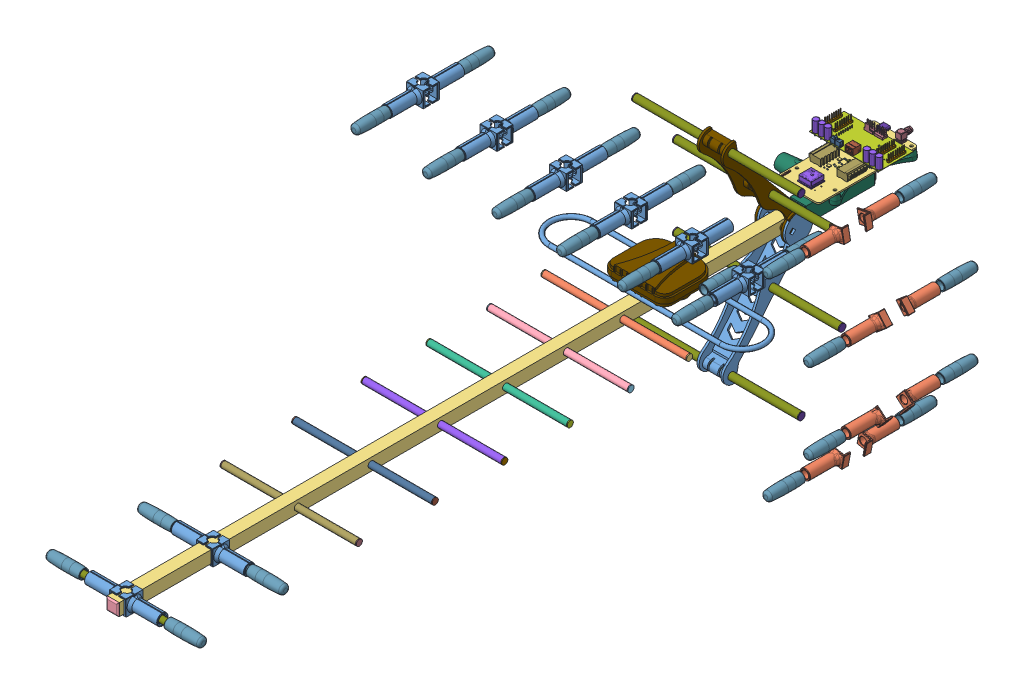
SolidWorks assembly 1. 868MHz Yagi Assembly, configuration Default. Lengths in mm. (continued)
Mates (geometry in assembly coordinates): (continued)
- Concentric20: concentric aligned: cylinder of naked_antenna_v1.step-1/2nd element.step-1/extrusion (2).step-1 through (440.0614 466.1407 645.9384) axis (0 0 1) radius 3.5; cylinder of antenna sheath-20 through (440.0614 466.1407 603.9384) axis (0 0 1) radius 4
- Concentric21: concentric aligned: cylinder of naked_antenna_v1.step-1/3rd element.step-1/extrusion (3).step-1 through (370.0614 466.1407 645.9384) axis (0 0 1) radius 3.5; cylinder of antenna sheath-21 through (370.0614 466.1407 603.9384) axis (0 0 1) radius 4
- Concentric22: concentric aligned: cylinder of naked_antenna_v1.step-1/3rd element.step-1/extrusion (3).step-1 through (370.0614 466.1407 645.9384) axis (0 0 1) radius 3.5; cylinder of antenna sheath-22 through (370.0614 466.1407 603.9384) axis (0 0 1) radius 4
- Concentric23: concentric aligned: cylinder of naked_antenna_v1.step-1/4th element.step-1/extrusion (4).step-1 through (295.0614 466.1407 645.9384) axis (0 0 1) radius 3.5; cylinder of antenna sheath-23 through (295.0614 466.1407 603.9384) axis (0 0 1) radius 4
- Concentric24: concentric aligned: cylinder of naked_antenna_v1.step-1/4th element.step-1/extrusion (4).step-1 through (295.0614 466.1407 645.9384) axis (0 0 1) radius 3.5; cylinder of antenna sheath-24 through (295.0614 466.1407 603.9384) axis (0 0 1) radius 4
- Concentric25: concentric aligned: cylinder of naked_antenna_v1.step-1/5th element.step-1/extrusion (5).step-1 through (215.0614 466.1407 645.9384) axis (0 0 1) radius 3.5; cylinder of antenna sheath-25 through (215.0614 466.1407 603.9384) axis (0 0 1) radius 4
- Concentric26: concentric aligned: cylinder of naked_antenna_v1.step-1/5th element.step-1/extrusion (5).step-1 through (215.0614 466.1407 645.9384) axis (0 0 1) radius 3.5; cylinder of antenna sheath-26 through (215.0614 466.1407 603.9384) axis (0 0 1) radius 4
- Concentric27: concentric aligned: cylinder of naked_antenna_v1.step-1/6th element.step-1/extrusion (6).step-1 through (130.0614 466.1407 645.9384) axis (0 0 1) radius 3.5; cylinder of antenna sheath-27 through (130.0614 466.1407 603.9384) axis (0 0 1) radius 4
- Concentric28: concentric aligned: cylinder of naked_antenna_v1.step-1/6th element.step-1/extrusion (6).step-1 through (130.0614 466.1407 645.9384) axis (0 0 1) radius 3.5; cylinder of antenna sheath-28 through (130.0614 466.1407 603.9384) axis (0 0 1) radius 4
- Concentric29: concentric aligned: cylinder of naked_antenna_v1.step-1/7th element.step-1/extrusion (7).step-1 through (40.0614 466.1407 645.9384) axis (0 0 1) radius 3.5; cylinder of antenna sheath-29 through (-42 0 757.5) axis (1 0 0) radius 4
- Concentric30: concentric aligned: cylinder of naked_antenna_v1.step-1/7th element.step-1/extrusion (7).step-1 through (40.0614 466.1407 645.9384) axis (0 0 1) radius 3.5; cylinder of antenna sheath-30 through (-42 0 757.5) axis (1 0 0) radius 4
- Concentric31: concentric aligned: cylinder of naked_antenna_v1.step-1/8th element.step-1/extrusion (8).step-1 through (-59.9386 466.1407 645.9384) axis (0 0 1) radius 3.5; cylinder of antenna sheath-31 through (-42 0 857.5) axis (1 0 0) radius 4
- Concentric32: concentric aligned: cylinder of naked_antenna_v1.step-1/8th element.step-1/extrusion (8).step-1 through (-59.9386 466.1407 645.9384) axis (0 0 1) radius 3.5; cylinder of antenna sheath-32 through (-42 0 857.5) axis (1 0 0) radius 4
- Coincident9: coincident anti-aligned: plane of naked_antenna_v1.step-1/Extrusion.step-1 through (754.5614 473.1407 652.9384) normal (0 0 1); plane of antenna sheath-3 through (440.0614 466.1407 652.9384) normal (0 0 -1)
- Coincident10: coincident anti-aligned: plane of naked_antenna_v1.step-1/Extrusion.step-1 through (754.5614 473.1407 652.9384) normal (0 0 1); plane of antenna sheath-4 through (440.0614 466.1407 652.9384) normal (0 0 -1)
- Coincident11: coincident anti-aligned: plane of naked_antenna_v1.step-1/Extrusion.step-1 through (754.5614 473.1407 652.9384) normal (0 0 1); plane of antenna sheath-5 through (370.0614 466.1407 652.9384) normal (0 0 -1)
- Coincident12: coincident anti-aligned: plane of naked_antenna_v1.step-1/Extrusion.step-1 through (754.5614 473.1407 652.9384) normal (0 0 1); plane of antenna sheath-6 through (370.0614 466.1407 652.9384) normal (0 0 -1)
- Coincident13: coincident anti-aligned: plane of naked_antenna_v1.step-1/Extrusion.step-1 through (754.5614 473.1407 652.9384) normal (0 0 1); plane of antenna sheath-7 through (295.0614 466.1407 652.9384) normal (0 0 -1)
- Coincident14: coincident anti-aligned: plane of naked_antenna_v1.step-1/Extrusion.step-1 through (754.5614 473.1407 652.9384) normal (0 0 1); plane of antenna sheath-8 through (295.0614 466.1407 652.9384) normal (0 0 -1)
- Coincident15: coincident anti-aligned: plane of naked_antenna_v1.step-1/Extrusion.step-1 through (754.5614 473.1407 652.9384) normal (0 0 1); plane of antenna sheath-9 through (215.0614 466.1407 652.9384) normal (0 0 -1)
- Coincident16: coincident anti-aligned: plane of naked_antenna_v1.step-1/Extrusion.step-1 through (754.5614 473.1407 652.9384) normal (0 0 1); plane of antenna sheath-10 through (215.0614 466.1407 652.9384) normal (0 0 -1)
- Coincident17: coincident anti-aligned: plane of naked_antenna_v1.step-1/Extrusion.step-1 through (754.5614 473.1407 652.9384) normal (0 0 1); plane of antenna sheath-11 through (130.0614 466.1407 652.9384) normal (0 0 -1)
- Coincident18: coincident anti-aligned: plane of naked_antenna_v1.step-1/Extrusion.step-1 through (754.5614 473.1407 652.9384) normal (0 0 1); plane of antenna sheath-12 through (130.0614 466.1407 652.9384) normal (0 0 -1)
- Coincident19: coincident anti-aligned: plane of naked_antenna_v1.step-1/Extrusion.step-1 through (754.5614 473.1407 652.9384) normal (0 0 1); plane of antenna sheath-13 through (40.0614 466.1407 652.9384) normal (0 0 -1)
- Coincident20: coincident anti-aligned: plane of naked_antenna_v1.step-1/Extrusion.step-1 through (754.5614 473.1407 652.9384) normal (0 0 1); plane of antenna sheath-14 through (40.0614 466.1407 652.9384) normal (0 0 -1)
- Coincident21: coincident anti-aligned: plane of naked_antenna_v1.step-1/Extrusion.step-1 through (754.5614 473.1407 652.9384) normal (0 0 1); plane of antenna sheath-15 through (-59.9386 466.1407 652.9384) normal (0 0 -1)
- Coincident22: coincident anti-aligned: plane of naked_antenna_v1.step-1/Extrusion.step-1 through (754.5614 473.1407 652.9384) normal (0 0 1); plane of antenna sheath-16 through (-59.9386 466.1407 652.9384) normal (0 0 -1)
- Coincident23: coincident anti-aligned: plane of naked_antenna_v1.step-1/Extrusion.step-1 through (754.5614 459.1407 638.9384) normal (0 0 -1); plane of antenna sheath-32 through (-59.9386 466.1407 638.9384) normal (0 0 1)
- Coincident24: coincident anti-aligned: plane of naked_antenna_v1.step-1/Extrusion.step-1 through (754.5614 459.1407 638.9384) normal (0 0 -1); plane of antenna sheath-31 through (-59.9386 466.1407 638.9384) normal (0 0 1)
- Coincident25: coincident anti-aligned: plane of naked_antenna_v1.step-1/Extrusion.step-1 through (754.5614 459.1407 638.9384) normal (0 0 -1); plane of antenna sheath-30 through (40.0614 466.1407 638.9384) normal (0 0 1)
- Coincident26: coincident anti-aligned: plane of naked_antenna_v1.step-1/Extrusion.step-1 through (754.5614 459.1407 638.9384) normal (0 0 -1); plane of antenna sheath-29 through (40.0614 466.1407 638.9384) normal (0 0 1)
- Coincident27: coincident anti-aligned: plane of naked_antenna_v1.step-1/Extrusion.step-1 through (754.5614 459.1407 638.9384) normal (0 0 -1); plane of antenna sheath-28 through (130.0614 466.1407 638.9384) normal (0 0 1)
- Coincident28: coincident anti-aligned: plane of naked_antenna_v1.step-1/Extrusion.step-1 through (754.5614 459.1407 638.9384) normal (0 0 -1); plane of antenna sheath-27 through (130.0614 466.1407 638.9384) normal (0 0 1)
- Coincident29: coincident anti-aligned: plane of naked_antenna_v1.step-1/Extrusion.step-1 through (754.5614 459.1407 638.9384) normal (0 0 -1); plane of antenna sheath-26 through (215.0614 466.1407 638.9384) normal (0 0 1)
- Coincident30: coincident anti-aligned: plane of naked_antenna_v1.step-1/Extrusion.step-1 through (754.5614 459.1407 638.9384) normal (0 0 -1); plane of antenna sheath-25 through (215.0614 466.1407 638.9384) normal (0 0 1)
- Coincident31: coincident anti-aligned: plane of naked_antenna_v1.step-1/Extrusion.step-1 through (754.5614 459.1407 638.9384) normal (0 0 -1); plane of antenna sheath-24 through (295.0614 466.1407 638.9384) normal (0 0 1)
- Coincident32: coincident anti-aligned: plane of naked_antenna_v1.step-1/Extrusion.step-1 through (754.5614 459.1407 638.9384) normal (0 0 -1); plane of antenna sheath-23 through (295.0614 466.1407 638.9384) normal (0 0 1)
- Coincident33: coincident anti-aligned: plane of naked_antenna_v1.step-1/Extrusion.step-1 through (754.5614 459.1407 638.9384) normal (0 0 -1); plane of antenna sheath-22 through (370.0614 466.1407 638.9384) normal (0 0 1)
- Coincident34: coincident anti-aligned: plane of naked_antenna_v1.step-1/Extrusion.step-1 through (754.5614 459.1407 638.9384) normal (0 0 -1); plane of antenna sheath-21 through (370.0614 466.1407 638.9384) normal (0 0 1)
- Coincident35: coincident anti-aligned: plane of naked_antenna_v1.step-1/Extrusion.step-1 through (754.5614 459.1407 638.9384) normal (0 0 -1); plane of antenna sheath-20 through (440.0614 466.1407 638.9384) normal (0 0 1)
- Coincident36: coincident anti-aligned: plane of naked_antenna_v1.step-1/Extrusion.step-1 through (754.5614 459.1407 638.9384) normal (0 0 -1); plane of antenna sheath-19 through (440.0614 466.1407 638.9384) normal (0 0 1)
- Parallel5: parallel anti-aligned: plane of naked_antenna_v1.step-1/Extrusion.step-1 through (754.5614 473.1407 638.9384) normal (0 1 0); plane of antenna sheath-4 through (440.0614 473.3907 646.9384) normal (0 -1 0)
- Parallel6: parallel anti-aligned: plane of naked_antenna_v1.step-1/Extrusion.step-1 through (754.5614 473.1407 638.9384) normal (0 1 0); plane of antenna sheath-3 through (430.0614 473.3907 646.9384) normal (0 -1 0)
- Parallel7: parallel anti-aligned: plane of naked_antenna_v1.step-1/Extrusion.step-1 through (754.5614 473.1407 638.9384) normal (0 1 0); plane of antenna sheath-20 through (450.0614 473.3907 644.9384) normal (0 -1 0)
- Parallel8: parallel anti-aligned: plane of naked_antenna_v1.step-1/Extrusion.step-1 through (754.5614 473.1407 638.9384) normal (0 1 0); plane of antenna sheath-19 through (440.0614 473.3907 644.9384) normal (0 -1 0)
- Parallel9: parallel anti-aligned: plane of naked_antenna_v1.step-1/Extrusion.step-1 through (754.5614 473.1407 638.9384) normal (0 1 0); plane of antenna sheath-21 through (370.0614 473.3907 644.9384) normal (0 -1 0)
- Parallel10: parallel anti-aligned: plane of naked_antenna_v1.step-1/Extrusion.step-1 through (754.5614 473.1407 638.9384) normal (0 1 0); plane of antenna sheath-22 through (380.0614 473.3907 644.9384) normal (0 -1 0)
- Parallel11: parallel anti-aligned: plane of naked_antenna_v1.step-1/Extrusion.step-1 through (754.5614 473.1407 638.9384) normal (0 1 0); plane of antenna sheath-6 through (360.0614 473.3907 646.9384) normal (0 -1 0)
- Parallel12: parallel anti-aligned: plane of naked_antenna_v1.step-1/Extrusion.step-1 through (754.5614 473.1407 638.9384) normal (0 1 0); plane of antenna sheath-5 through (370.0614 473.3907 646.9384) normal (0 -1 0)
- Parallel13: parallel anti-aligned: plane of naked_antenna_v1.step-1/Extrusion.step-1 through (754.5614 473.1407 638.9384) normal (0 1 0); plane of antenna sheath-8 through (295.0614 473.3907 646.9384) normal (0 -1 0)
- Parallel14: parallel anti-aligned: plane of naked_antenna_v1.step-1/Extrusion.step-1 through (754.5614 473.1407 638.9384) normal (0 1 0); plane of antenna sheath-7 through (285.0614 473.3907 646.9384) normal (0 -1 0)
- Parallel15: parallel anti-aligned: plane of naked_antenna_v1.step-1/Extrusion.step-1 through (754.5614 473.1407 638.9384) normal (0 1 0); plane of antenna sheath-23 through (305.0614 473.3907 644.9384) normal (0 -1 0)
- Parallel16: parallel anti-aligned: plane of naked_antenna_v1.step-1/Extrusion.step-1 through (754.5614 473.1407 638.9384) normal (0 1 0); plane of antenna sheath-24 through (295.0614 473.3907 644.9384) normal (0 -1 0)
- Parallel17: parallel anti-aligned: plane of naked_antenna_v1.step-1/Extrusion.step-1 through (754.5614 473.1407 638.9384) normal (0 1 0); plane of antenna sheath-9 through (205.0614 473.3907 646.9384) normal (0 -1 0)
- Parallel18: parallel anti-aligned: plane of naked_antenna_v1.step-1/Extrusion.step-1 through (754.5614 473.1407 638.9384) normal (0 1 0); plane of antenna sheath-10 through (215.0614 473.3907 646.9384) normal (0 -1 0)
- Parallel19: parallel anti-aligned: plane of naked_antenna_v1.step-1/Extrusion.step-1 through (754.5614 473.1407 638.9384) normal (0 1 0); plane of antenna sheath-25 through (215.0614 473.3907 644.9384) normal (0 -1 0)
- Parallel20: parallel anti-aligned: plane of naked_antenna_v1.step-1/Extrusion.step-1 through (754.5614 473.1407 638.9384) normal (0 1 0); plane of antenna sheath-26 through (225.0614 473.3907 644.9384) normal (0 -1 0)
- Parallel21: parallel anti-aligned: plane of naked_antenna_v1.step-1/Extrusion.step-1 through (754.5614 473.1407 638.9384) normal (0 1 0); plane of antenna sheath-12 through (130.0614 473.3907 646.9384) normal (0 -1 0)
- Parallel22: parallel anti-aligned: plane of naked_antenna_v1.step-1/Extrusion.step-1 through (754.5614 473.1407 638.9384) normal (0 1 0); plane of antenna sheath-11 through (120.0614 473.3907 646.9384) normal (0 -1 0)
- Parallel23: parallel anti-aligned: plane of naked_antenna_v1.step-1/Extrusion.step-1 through (754.5614 473.1407 638.9384) normal (0 1 0); plane of antenna sheath-27 through (140.0614 473.3907 644.9384) normal (0 -1 0)
- Parallel24: parallel anti-aligned: plane of naked_antenna_v1.step-1/Extrusion.step-1 through (754.5614 473.1407 638.9384) normal (0 1 0); plane of antenna sheath-28 through (130.0614 473.3907 644.9384) normal (0 -1 0)
- Parallel25: parallel anti-aligned: plane of naked_antenna_v1.step-1/Extrusion.step-1 through (754.5614 473.1407 638.9384) normal (0 1 0); plane of antenna sheath-14 through (40.0614 473.3907 646.9384) normal (0 -1 0)
- Parallel26: parallel anti-aligned: plane of naked_antenna_v1.step-1/Extrusion.step-1 through (754.5614 473.1407 638.9384) normal (0 1 0); plane of antenna sheath-13 through (30.0614 473.3907 646.9384) normal (0 -1 0)
- Parallel27: parallel anti-aligned: plane of naked_antenna_v1.step-1/Extrusion.step-1 through (754.5614 473.1407 638.9384) normal (0 1 0); plane of antenna sheath-30 through (40.0614 473.3907 644.9384) normal (0 -1 0)
- Parallel28: parallel anti-aligned: plane of naked_antenna_v1.step-1/Extrusion.step-1 through (754.5614 473.1407 638.9384) normal (0 1 0); plane of antenna sheath-29 through (50.0614 473.3907 644.9384) normal (0 -1 0)
- Parallel29: parallel anti-aligned: plane of naked_antenna_v1.step-1/Extrusion.step-1 through (754.5614 473.1407 638.9384) normal (0 1 0); plane of antenna sheath-16 through (-69.9386 473.3907 646.9384) normal (0 -1 0)
- Parallel30: parallel anti-aligned: plane of naked_antenna_v1.step-1/Extrusion.step-1 through (754.5614 473.1407 638.9384) normal (0 1 0); plane of antenna sheath-15 through (-59.9386 473.3907 646.9384) normal (0 -1 0)
- Parallel31: parallel anti-aligned: plane of naked_antenna_v1.step-1/Extrusion.step-1 through (754.5614 473.1407 638.9384) normal (0 1 0); plane of antenna sheath-32 through (-59.9386 473.3907 644.9384) normal (0 -1 0)
- Parallel32: parallel anti-aligned: plane of naked_antenna_v1.step-1/Extrusion.step-1 through (754.5614 473.1407 638.9384) normal (0 1 0); plane of antenna sheath-31 through (-49.9386 473.3907 644.9384) normal (0 -1 0)
- Concentric33: concentric anti-aligned: cylinder of naked_antenna_v1.step-1/Reflector.step-1/struct_1.step-1/element_2.step-1/extrusion_1.step-1 through (622.1186 354.933 645.9384) axis (0 0 -1) radius 4; cylinder of ground plane sheath-1 through (622.1186 354.933 593.9384) axis (0 0 1) radius 4
- Parallel33: parallel anti-aligned: plane of naked_antenna_v1.step-1/Reflector.step-1/struct_1.step-1/struct_1-1.step-1 through (627.0129 345.8613 630.9384) normal (0.982463 -0.186459 0); plane of ground plane sheath-1 through (630.3943 360.9962 636.9384) normal (-0.982463 0.186459 0)
- Coincident66: coincident anti-aligned: plane of naked_antenna_v1.step-1/Reflector.step-1/struct_1.step-1/struct_1-1.step-1 through (663.0058 413.8665 630.9384) normal (0 0 -1); plane of ground plane sheath-1 through (622.1186 354.933 630.9384) normal (0 0 1)
- Concentric34: concentric aligned: cylinder of naked_antenna_v1.step-1/Reflector.step-1/struct_1.step-1/element_2.step-1/extrusion_1.step-1 through (622.1186 354.933 645.9384) axis (0 0 -1) radius 4; cylinder of ground plane sheath-2 through (622.1186 354.933 697.9384) axis (0 0 -1) radius 4
- Coincident67: coincident anti-aligned: plane of naked_antenna_v1.step-1/Reflector.step-1/struct_1.step-1/struct_1-1.step-1 through (658.3878 400.0587 660.9384) normal (0 0 1); plane of ground plane sheath-2 through (622.1186 354.933 660.9384) normal (0 0 -1)
- Parallel34: parallel anti-aligned: plane of naked_antenna_v1.step-1/Reflector.step-1/struct_1.step-1/struct_1-1.step-1 through (627.0129 345.8613 630.9384) normal (0.982463 -0.186459 0); plane of ground plane sheath-2 through (627.5974 346.2593 654.9384) normal (-0.982463 0.186459 0)
- Concentric35: concentric aligned: cylinder of naked_antenna_v1.step-1/Reflector.step-1/struct_1.step-1/element_3.step-1/extrusion_1.step-1 through (669.0995 419.8148 645.9384) axis (0 0 -1) radius 4; cylinder of ground plane sheath-3 through (669.0995 419.8148 697.9384) axis (0 0 -1) radius 4
- Coincident69: coincident anti-aligned: plane of naked_antenna_v1.step-1/Reflector.step-1/struct_1.step-1/struct_1-1.step-1 through (658.3878 400.0587 660.9384) normal (0 0 1); plane of ground plane sheath-3 through (669.0995 419.8148 660.9384) normal (0 0 -1)
- Parallel35: parallel anti-aligned: plane of naked_antenna_v1.step-1/Reflector.step-1/struct_1.step-1/struct_1-1.step-1 through (630.3692 363.5456 630.9384) normal (0.766044 -0.642788 0); plane of ground plane sheath-3 through (669.6409 409.5699 654.9384) normal (-0.766044 0.642788 0)
- Concentric36: concentric anti-aligned: cylinder of naked_antenna_v1.step-1/Reflector.step-1/struct_1.step-1/element_3.step-1/extrusion_1.step-1 through (669.0995 419.8148 645.9384) axis (0 0 -1) radius 4; cylinder of ground plane sheath-4 through (669.0995 419.8148 593.9384) axis (0 0 1) radius 4
- Coincident71: coincident anti-aligned: plane of naked_antenna_v1.step-1/Reflector.step-1/struct_1.step-1/struct_1-1.step-1 through (663.0058 413.8665 630.9384) normal (0 0 -1); plane of ground plane sheath-4 through (669.0995 419.8148 630.9384) normal (0 0 1)
- Parallel36: parallel anti-aligned: plane of naked_antenna_v1.step-1/Reflector.step-1/struct_1.step-1/struct_1-1.step-1 through (630.3692 363.5456 630.9384) normal (0.766044 -0.642788 0); plane of ground plane sheath-4 through (679.2827 421.0606 636.9384) normal (-0.766044 0.642788 0)
- Concentric37: concentric aligned: cylinder of naked_antenna_v1.step-1/Reflector.step-1/struct.step-1/element_1.step-1/extrusion_1.step-1 through (669.0995 512.4667 645.9384) axis (0 0 1) radius 4; cylinder of ground plane sheath-6 through (669.0995 512.4667 593.9384) axis (0 0 1) radius 4
- Parallel37: parallel anti-aligned: plane of naked_antenna_v1.step-1/Reflector.step-1/struct.step-1/struct-0.step-1 through (630.3692 568.7358 660.9384) normal (0.766044 0.642788 0); plane of ground plane sheath-6 through (669.6409 522.7116 636.9384) normal (-0.766044 -0.642788 0)
- Coincident74: coincident anti-aligned: plane of naked_antenna_v1.step-1/Reflector.step-1/struct.step-1/struct-0.step-1 through (658.3878 532.2228 630.9384) normal (0 0 -1); plane of ground plane sheath-6 through (669.0995 512.4667 630.9384) normal (0 0 1)
- Concentric38: concentric aligned: cylinder of naked_antenna_v1.step-1/Reflector.step-1/struct.step-1/element.step-1/extrusion_1.step-1 through (622.1186 577.3485 645.9384) axis (0 0 1) radius 4; cylinder of ground plane sheath-8 through (622.1186 577.3485 593.9384) axis (0 0 1) radius 4
- Coincident75: coincident anti-aligned: plane of naked_antenna_v1.step-1/Reflector.step-1/struct.step-1/struct-0.step-1 through (658.3878 532.2228 630.9384) normal (0 0 -1); plane of ground plane sheath-8 through (622.1186 577.3485 630.9384) normal (0 0 1)
- Parallel38: parallel anti-aligned: plane of naked_antenna_v1.step-1/Reflector.step-1/struct.step-1/struct-0.step-1 through (627.0129 586.4202 660.9384) normal (0.982463 0.186459 0); plane of ground plane sheath-8 through (627.5974 586.0222 636.9384) normal (-0.982463 -0.186459 0)
- Concentric39: concentric anti-aligned: cylinder of naked_antenna_v1.step-1/Reflector.step-1/struct.step-1/element.step-1/extrusion_1.step-1 through (622.1186 577.3485 645.9384) axis (0 0 1) radius 4; cylinder of ground plane sheath-7 through (622.1186 577.3485 697.9384) axis (0 0 -1) radius 4
- Coincident77: coincident anti-aligned: plane of naked_antenna_v1.step-1/Reflector.step-1/struct.step-1/struct-0.step-1 through (663.0058 518.415 660.9384) normal (0 0 1); plane of ground plane sheath-7 through (622.1186 577.3485 660.9384) normal (0 0 -1)
- Parallel39: parallel anti-aligned: plane of naked_antenna_v1.step-1/Reflector.step-1/struct.step-1/struct-0.step-1 through (627.0129 586.4202 660.9384) normal (0.982463 0.186459 0); plane of ground plane sheath-7 through (630.3943 571.2852 654.9384) normal (-0.982463 -0.186459 0)
- Concentric40: concentric anti-aligned: cylinder of naked_antenna_v1.step-1/Reflector.step-1/struct.step-1/element_1.step-1/extrusion_1.step-1 through (669.0995 512.4667 645.9384) axis (0 0 1) radius 4; cylinder of ground plane sheath-5 through (669.0995 512.4667 697.9384) axis (0 0 -1) radius 4
- Parallel40: parallel anti-aligned: plane of naked_antenna_v1.step-1/Reflector.step-1/struct.step-1/struct-0.step-1 through (630.3692 568.7358 660.9384) normal (0.766044 0.642788 0); plane of ground plane sheath-5 through (679.2827 511.2209 654.9384) normal (-0.766044 -0.642788 0)
- Coincident80: coincident anti-aligned: plane of naked_antenna_v1.step-1/Reflector.step-1/struct.step-1/struct-0.step-1 through (663.0058 518.415 660.9384) normal (0 0 1); plane of ground plane sheath-5 through (669.0995 512.4667 660.9384) normal (0 0 -1)
- Width1: width anti-aligned: plane of Yagi Adaptor-1 through (-7.25 7.25 84.0355) normal (0 -1 0); plane of naked_antenna_v1.step-1/Extrusion.step-1 through (-7.25 -7.25 84.0355) normal (0 1 0); plane of Yagi Adaptor-1 through (754.5614 473.1407 638.9384) normal (0 1 0); plane of naked_antenna_v1.step-1/Extrusion.step-1 through (754.5614 459.1407 652.9384) normal (0 -1 0)
- Width2: width aligned: plane of Yagi Adaptor-1 through (7.25 7.25 84.0355) normal (-1 0 0); plane of naked_antenna_v1.step-1/Extrusion.step-1 through (-7.25 7.25 84.0355) normal (1 0 0); plane of Yagi Adaptor-1 through (754.5614 459.1407 638.9384) normal (0 0 -1); plane of naked_antenna_v1.step-1/Extrusion.step-1 through (754.5614 473.1407 652.9384) normal (0 0 1)
- Tangent1: tangent anti-aligned: cylinder of naked_antenna_v1.step-1/Reflector.step-1/struct_1.step-1/struct_1-1.step-1 through (697.5259 466.1407 630.9384) axis (0 0 1) radius 16; plane of Yagi Adaptor-1 through (0 0 84.0355) normal (0 0 1)
- Concentric41: concentric aligned: cylinder of Yagi Adaptor-1 through (22 11.75 63.0355) axis (0 -1 0) radius 1.75; cylinder of Main_Board_1_1-1/Main_Board_1_1_BOARD-1 through (22 19.75 63.0355) axis (0 -1 0) radius 1.6
- Concentric42: concentric aligned: cylinder of Yagi Adaptor-1 through (22 11.75 -24.9645) axis (0 -1 0) radius 1.75; cylinder of Main_Board_1_1-1/Main_Board_1_1_BOARD-1 through (22 19.75 -24.9645) axis (0 -1 0) radius 1.6
- Coincident83: coincident anti-aligned: plane of Yagi Adaptor-1 through (-25.25 19.75 63.0355) normal (0 1 0); plane of Main_Board_1_1-1/Main_Board_1_1_BOARD-1 through (22.8 19.75 -25.7645) normal (0 -1 0)
- Coincident84: coincident anti-aligned: plane of Main_Board_1_1-1/SLIN-PPPC081LFBN-RC_V_CMP-002-00028-2-2 through (-19.4499 29.0021 19.4712) normal (1 0 0); plane of Ground_Station_-_Copy_for_Callum_and_Yiannis-1/FP-M20-9990846-MFG_CMP-15831-000033-1-1 through (-19.4499 29.8565 20.3256) normal (-1 0 0)
- Coincident85: coincident anti-aligned: plane of Main_Board_1_1-1/SLIN-PPPC081LFBN-RC_V_CMP-002-00028-2-2 through (-19.5043 29.0021 20.3256) normal (0 0 -1); plane of Ground_Station_-_Copy_for_Callum_and_Yiannis-1/FP-M20-9990846-MFG_CMP-15831-000033-1-1 through (-18.8099 29.8565 20.3256) normal (0 0 1)
- Coincident86: coincident anti-aligned: plane of Main_Board_1_1-1/SLIN-PPPC081LFBN-RC_V_CMP-002-00028-2-2 through (-17.7255 29.8565 22.2684) normal (0 1 0); plane of Ground_Station_-_Copy_for_Callum_and_Yiannis-1/FP-M20-9990846-MFG_CMP-15831-000033-1-1 through (-19.1299 29.8565 20.0056) normal (0 -1 0)
- Concentric43: concentric anti-aligned: cylinder of naked_antenna_v1.step-1/8th element.step-1/extrusion (8).step-1 through (-59.9386 466.1407 645.9384) axis (0 0 1) radius 3.5; cylinder of 868MHz Yagi Tip Covers-1 through (-49 0 857.5) axis (-1 0 0) radius 4.25
- Coincident87: coincident anti-aligned: plane of naked_antenna_v1.step-1/8th element.step-1/end cap (8).step-2 through (-59.9386 466.1407 561.9384) normal (0 0 -1); plane of 868MHz Yagi Tip Covers-1 through (-84 0 857.5) normal (1 0 0)
- Concentric44: concentric anti-aligned: cylinder of naked_antenna_v1.step-1/7th element.step-1/extrusion (7).step-1 through (40.0614 466.1407 645.9384) axis (0 0 1) radius 3.5; cylinder of 868MHz Yagi Tip Covers-22 through (-43.5 0 757.5) axis (-1 0 0) radius 4.25
- Concentric45: concentric anti-aligned: cylinder of naked_antenna_v1.step-1/5th element.step-1/extrusion (5).step-1 through (215.0614 466.1407 645.9384) axis (0 0 1) radius 3.5; cylinder of 868MHz Yagi Tip Covers-20 through (215.0614 466.1407 603.9384) axis (0 0 -1) radius 4.25
- Concentric46: concentric: cylinder of naked_antenna_v1.step-1/4th element.step-1/extrusion (4).step-1 through (295.0614 466.1407 645.9384) axis (0 0 1) radius 3.5; cylinder of 868MHz Yagi Tip Covers-19 through (295.0614 466.1407 603.9384) axis (0 0 -1) radius 4.25
- Concentric47: concentric: cylinder of naked_antenna_v1.step-1/3rd element.step-1/extrusion (3).step-1 through (370.0614 466.1407 645.9384) axis (0 0 1) radius 3.5; cylinder of 868MHz Yagi Tip Covers-18 through (370.0614 466.1407 603.4384) axis (0 0 -1) radius 4.25
- Concentric48: concentric: cylinder of naked_antenna_v1.step-1/2nd element.step-1/extrusion (2).step-1 through (440.0614 466.1407 645.9384) axis (0 0 1) radius 3.5; cylinder of 868MHz Yagi Tip Covers-17 through (475.435 450.7404 667.737) axis (0 0 -1) radius 4.25
- Concentric49: concentric: cylinder of naked_antenna_v1.step-1/1st element.step-1/extrusion (1).step-1 through (505.0614 466.1407 645.9384) axis (0 0 1) radius 3.5; cylinder of 868MHz Yagi Tip Covers-16 through (505.0614 466.1407 600.9384) axis (0 0 -1) radius 4.25
- Concentric50: concentric: cylinder of naked_antenna_v1.step-1/Reflector.step-1/struct.step-1/element_1.step-1/extrusion_1.step-1 through (669.0995 512.4667 645.9384) axis (0 0 1) radius 4; cylinder of 868MHz Yagi Tip Covers-15 through (669.0995 512.4667 588.9384) axis (0 0 -1) radius 4.25
- Concentric51: concentric: cylinder of naked_antenna_v1.step-1/Reflector.step-1/struct.step-1/element.step-1/extrusion_1.step-1 through (622.1186 577.3485 645.9384) axis (0 0 1) radius 4; cylinder of 868MHz Yagi Tip Covers-14 through (622.1186 577.3485 588.9384) axis (0 0 -1) radius 4.25
- Concentric52: concentric: cylinder of naked_antenna_v1.step-1/Reflector.step-1/struct.step-1/element.step-1/extrusion_1.step-1 through (622.1186 577.3485 645.9384) axis (0 0 1) radius 4; cylinder of 868MHz Yagi Tip Covers-13 through (622.1186 577.3485 702.9384) axis (0 0 1) radius 4.25
- Concentric53: concentric: cylinder of naked_antenna_v1.step-1/Reflector.step-1/struct.step-1/element_1.step-1/extrusion_1.step-1 through (669.0995 512.4667 645.9384) axis (0 0 1) radius 4; cylinder of 868MHz Yagi Tip Covers-12 through (669.0995 512.4667 702.9384) axis (0 0 1) radius 4.25
- Concentric54: concentric: cylinder of naked_antenna_v1.step-1/Reflector.step-1/struct_1.step-1/element_3.step-1/extrusion_1.step-1 through (669.0995 419.8148 645.9384) axis (0 0 -1) radius 4; cylinder of 868MHz Yagi Tip Covers-11 through (669.0995 419.8148 702.9384) axis (0 0 1) radius 4.25
- Concentric55: concentric: cylinder of naked_antenna_v1.step-1/Reflector.step-1/struct_1.step-1/element_2.step-1/extrusion_1.step-1 through (622.1186 354.933 645.9384) axis (0 0 -1) radius 4; cylinder of 868MHz Yagi Tip Covers-10 through (622.1186 354.933 702.9384) axis (0 0 1) radius 4.25
- Concentric56: concentric: cylinder of naked_antenna_v1.step-1/1st element.step-1/extrusion (1).step-1 through (505.0614 466.1407 645.9384) axis (0 0 1) radius 3.5; cylinder of 868MHz Yagi Tip Covers-9 through (505.0614 466.1407 690.9384) axis (0 0 1) radius 4.25
- Concentric57: concentric: cylinder of naked_antenna_v1.step-1/2nd element.step-1/extrusion (2).step-1 through (440.0614 466.1407 645.9384) axis (0 0 1) radius 3.5; cylinder of 868MHz Yagi Tip Covers-8 through (440.0614 466.1407 688.4384) axis (0 0 1) radius 4.25
- Concentric58: concentric: cylinder of naked_antenna_v1.step-1/3rd element.step-1/extrusion (3).step-1 through (370.0614 466.1407 645.9384) axis (0 0 1) radius 3.5; cylinder of 868MHz Yagi Tip Covers-7 through (370.0614 466.1407 688.4384) axis (0 0 1) radius 4.25
- Concentric59: concentric: cylinder of naked_antenna_v1.step-1/4th element.step-1/extrusion (4).step-1 through (295.0614 466.1407 645.9384) axis (0 0 1) radius 3.5; cylinder of 868MHz Yagi Tip Covers-6 through (295.0614 466.1407 687.9384) axis (0 0 1) radius 4.25
- Concentric60: concentric: cylinder of naked_antenna_v1.step-1/5th element.step-1/extrusion (5).step-1 through (215.0614 466.1407 645.9384) axis (0 0 1) radius 3.5; cylinder of 868MHz Yagi Tip Covers-5 through (215.0614 466.1407 687.9384) axis (0 0 1) radius 4.25
- Concentric61: concentric: cylinder of naked_antenna_v1.step-1/6th element.step-1/extrusion (6).step-1 through (130.0614 466.1407 645.9384) axis (0 0 1) radius 3.5; cylinder of 868MHz Yagi Tip Covers-4 through (130.0614 466.1407 685.4384) axis (0 0 1) radius 4.25
- Concentric62: concentric: cylinder of naked_antenna_v1.step-1/7th element.step-1/extrusion (7).step-1 through (40.0614 466.1407 645.9384) axis (0 0 1) radius 3.5; cylinder of 868MHz Yagi Tip Covers-3 through (43.5 0 757.5) axis (1 0 0) radius 4.25
- Concentric63: concentric: cylinder of naked_antenna_v1.step-1/8th element.step-1/extrusion (8).step-1 through (-59.9386 466.1407 645.9384) axis (0 0 1) radius 3.5; cylinder of 868MHz Yagi Tip Covers-2 through (49 0 857.5) axis (1 0 0) radius 4.25
- Concentric65: concentric anti-aligned: cylinder of naked_antenna_v1.step-1/6th element.step-1/extrusion (6).step-1 through (130.0614 466.1407 645.9384) axis (0 0 1) radius 3.5; cylinder of 868MHz Yagi Tip Covers-21 through (130.0614 466.1407 606.4384) axis (0 0 -1) radius 4.25
- Coincident89: coincident anti-aligned: plane of naked_antenna_v1.step-1/7th element.step-1/end cap (7).step-2 through (40.0614 466.1407 567.4384) normal (0 0 -1); plane of 868MHz Yagi Tip Covers-22 through (-78.5 0 757.5) normal (1 0 0)
- Coincident90: coincident anti-aligned: plane of naked_antenna_v1.step-1/6th element.step-1/end cap (6).step-2 through (130.0614 466.1407 567.4384) normal (0 0 -1); plane of 868MHz Yagi Tip Covers-21 through (130.0614 466.1407 571.4384) normal (0 0 1)
- Coincident91: coincident anti-aligned: plane of naked_antenna_v1.step-1/5th element.step-1/end cap (5).step-2 through (215.0614 466.1407 564.9384) normal (0 0 -1); plane of 868MHz Yagi Tip Covers-20 through (215.0614 466.1407 568.9384) normal (0 0 1)
- Coincident93: coincident anti-aligned: plane of naked_antenna_v1.step-1/4th element.step-1/end cap (4).step-2 through (295.0614 466.1407 564.9384) normal (0 0 -1); plane of 868MHz Yagi Tip Covers-19 through (295.0614 466.1407 568.9384) normal (0 0 1)
- Coincident94: coincident anti-aligned: plane of naked_antenna_v1.step-1/3rd element.step-1/end cap (3).step-2 through (370.0614 466.1407 564.4384) normal (0 0 -1); plane of 868MHz Yagi Tip Covers-18 through (370.0614 466.1407 568.4384) normal (0 0 1)
- Coincident95: coincident anti-aligned: plane of naked_antenna_v1.step-1/2nd element.step-1/end cap (2).step-2 through (440.0614 466.1407 564.4384) normal (0 0 -1); plane of 868MHz Yagi Tip Covers-17 through (475.435 450.7404 632.737) normal (0 0 1)
- Coincident96: coincident anti-aligned: plane of naked_antenna_v1.step-1/1st element.step-1/end cap (1).step-2 through (505.0614 466.1407 561.9384) normal (0 0 -1); plane of 868MHz Yagi Tip Covers-16 through (505.0614 466.1407 565.9384) normal (0 0 1)
- Coincident97: coincident anti-aligned: plane of naked_antenna_v1.step-1/Reflector.step-1/struct.step-1/element.step-1/end cap_1.step-2 through (622.1186 577.3485 549.9384) normal (0 0 -1); plane of 868MHz Yagi Tip Covers-14 through (622.1186 577.3485 553.9384) normal (0 0 1)
- Coincident98: coincident anti-aligned: plane of naked_antenna_v1.step-1/Reflector.step-1/struct.step-1/element_1.step-1/end cap_1.step-2 through (669.0995 512.4667 549.9384) normal (0 0 -1); plane of 868MHz Yagi Tip Covers-15 through (669.0995 512.4667 553.9384) normal (0 0 1)
- Coincident99: coincident anti-aligned: plane of naked_antenna_v1.step-1/Reflector.step-1/struct_1.step-1/element_2.step-1/end cap_1.step-2 through (622.1186 354.933 741.9384) normal (0 0 1); plane of 868MHz Yagi Tip Covers-10 through (622.1186 354.933 737.9384) normal (0 0 -1)
- Coincident100: coincident anti-aligned: plane of naked_antenna_v1.step-1/Reflector.step-1/struct_1.step-1/element_3.step-1/end cap_1.step-2 through (669.0995 419.8148 741.9384) normal (0 0 1); plane of 868MHz Yagi Tip Covers-11 through (669.0995 419.8148 737.9384) normal (0 0 -1)
- Coincident101: coincident anti-aligned: plane of naked_antenna_v1.step-1/Reflector.step-1/struct.step-1/element_1.step-1/end cap_1.step-1 through (669.0995 512.4667 741.9384) normal (0 0 1); plane of 868MHz Yagi Tip Covers-12 through (669.0995 512.4667 737.9384) normal (0 0 -1)
- Coincident102: coincident anti-aligned: plane of naked_antenna_v1.step-1/Reflector.step-1/struct.step-1/element.step-1/end cap_1.step-1 through (622.1186 577.3485 741.9384) normal (0 0 1); plane of 868MHz Yagi Tip Covers-13 through (622.1186 577.3485 737.9384) normal (0 0 -1)
- Coincident103: coincident anti-aligned: plane of naked_antenna_v1.step-1/1st element.step-1/end cap (1).step-1 through (505.0614 466.1407 729.9384) normal (0 0 1); plane of 868MHz Yagi Tip Covers-9 through (505.0614 466.1407 725.9384) normal (0 0 -1)
- Coincident104: coincident anti-aligned: plane of naked_antenna_v1.step-1/2nd element.step-1/end cap (2).step-1 through (440.0614 466.1407 727.4384) normal (0 0 1); plane of 868MHz Yagi Tip Covers-8 through (440.0614 466.1407 723.4384) normal (0 0 -1)
- Coincident105: coincident anti-aligned: plane of naked_antenna_v1.step-1/3rd element.step-1/end cap (3).step-1 through (370.0614 466.1407 727.4384) normal (0 0 1); plane of 868MHz Yagi Tip Covers-7 through (370.0614 466.1407 723.4384) normal (0 0 -1)
- Coincident106: coincident anti-aligned: plane of naked_antenna_v1.step-1/4th element.step-1/end cap (4).step-1 through (295.0614 466.1407 726.9384) normal (0 0 1); plane of 868MHz Yagi Tip Covers-6 through (295.0614 466.1407 722.9384) normal (0 0 -1)
- Coincident107: coincident anti-aligned: plane of naked_antenna_v1.step-1/5th element.step-1/end cap (5).step-1 through (215.0614 466.1407 726.9384) normal (0 0 1); plane of 868MHz Yagi Tip Covers-5 through (215.0614 466.1407 722.9384) normal (0 0 -1)
- Coincident108: coincident anti-aligned: plane of naked_antenna_v1.step-1/6th element.step-1/end cap (6).step-1 through (130.0614 466.1407 724.4384) normal (0 0 1); plane of 868MHz Yagi Tip Covers-4 through (130.0614 466.1407 720.4384) normal (0 0 -1)
- Coincident109: coincident anti-aligned: plane of naked_antenna_v1.step-1/7th element.step-1/end cap (7).step-1 through (40.0614 466.1407 724.4384) normal (0 0 1); plane of 868MHz Yagi Tip Covers-3 through (78.5 0 757.5) normal (-1 0 0)
- Coincident110: coincident anti-aligned: plane of naked_antenna_v1.step-1/8th element.step-1/end cap (8).step-1 through (-59.9386 466.1407 729.9384) normal (0 0 1); plane of 868MHz Yagi Tip Covers-2 through (84 0 857.5) normal (-1 0 0)
- Concentric66: concentric: cylinder of naked_antenna_v1.step-1/Reflector.step-1/struct_1.step-1/element_3.step-1/extrusion_1.step-1 through (669.0995 419.8148 645.9384) axis (0 0 -1) radius 4; cylinder of 868MHz Yagi Tip Covers-23 through (669.0995 419.8148 553.9384) axis (0 0 -1) radius 6
- Coincident111: coincident anti-aligned: plane of naked_antenna_v1.step-1/Reflector.step-1/struct_1.step-1/element_3.step-1/end cap_1.step-1 through (669.0995 419.8148 549.9384) normal (0 0 -1); plane of 868MHz Yagi Tip Covers-23 through (669.0995 419.8148 553.9384) normal (0 0 1)
- Concentric67: concentric: cylinder of naked_antenna_v1.step-1/Reflector.step-1/struct_1.step-1/element_2.step-1/extrusion_1.step-1 through (622.1186 354.933 645.9384) axis (0 0 -1) radius 4; cylinder of 868MHz Yagi Tip Covers-24 through (622.1186 354.933 553.9384) axis (0 0 -1) radius 6
- Coincident112: coincident anti-aligned: plane of naked_antenna_v1.step-1/Reflector.step-1/struct_1.step-1/element_2.step-1/end cap_1.step-1 through (622.1186 354.933 549.9384) normal (0 0 -1); plane of 868MHz Yagi Tip Covers-24 through (622.1186 354.933 553.9384) normal (0 0 1)
- Coincident114: coincident: point of naked_antenna_v1-1/naked_antenna_v1.step-1/Extrusion.step-1
- Coincident116: coincident anti-aligned: plane of naked_antenna_v1-1/naked_antenna_v1.step-1/End Cap.step-1 through (0 0 0) normal (0 0 -1)
- Width4: width anti-aligned: plane of Yagi Adaptor-1 through (7.25 7.25 84.0355) normal (-1 0 0); plane of naked_antenna_v1-1/naked_antenna_v1.step-1/Extrusion.step-1 through (-7.25 7.25 84.0355) normal (1 0 0); plane of Yagi Adaptor-1 through (7 7 43) normal (1 0 0); plane of naked_antenna_v1-1/naked_antenna_v1.step-1/Extrusion.step-1 through (-7 -7 43) normal (-1 0 0)
- Width5: width anti-aligned: plane of Yagi Adaptor-1 through (-7.25 -7.25 84.0355) normal (0 1 0); plane of naked_antenna_v1-1/naked_antenna_v1.step-1/Extrusion.step-1 through (-7.25 7.25 84.0355) normal (0 -1 0); plane of Yagi Adaptor-1 through (7 -7 43) normal (0 -1 0); plane of naked_antenna_v1-1/naked_antenna_v1.step-1/Extrusion.step-1 through (-7 7 43) normal (0 1 0)
- Tangent2: tangent anti-aligned: plane of Yagi Adaptor-1 through (0 0 84.0355) normal (0 0 1); cylinder of naked_antenna_v1-1/naked_antenna_v1.step-1/Reflector.step-1/struct.step-1/struct-0.step-1 through (15 0 100.0355) axis (-1 0 0) radius 16
- Concentric68: concentric anti-aligned: cylinder of 868MHz Yagi Tip Covers-1 through (-84 0 857.5) axis (-1 0 0) radius 6; cylinder of naked_antenna_v1-1/naked_antenna_v1.step-1/8th element.step-1/extrusion (8).step-1 through (0 0 857.5) axis (1 0 0) radius 3.5
- Coincident117: coincident: unknown of Yagi Adaptor-1
- Parallel41: parallel aligned: plane of naked_antenna_v1-1/naked_antenna_v1.step-1/Extrusion.step-1 through (-7 7 43) normal (0 1 0)
- Coincident119: coincident anti-aligned: plane of 868MHz Yagi Tip Covers-1 through (-84 0 857.5) normal (1 0 0); plane of naked_antenna_v1-1/naked_antenna_v1.step-1/8th element.step-1/end cap (8).step-2 through (-84 0 857.5) normal (-1 0 0)
- Concentric69: concentric aligned: cylinder of antenna sheath-32 through (-42 0 857.5) axis (1 0 0) radius 4; cylinder of naked_antenna_v1-1/naked_antenna_v1.step-1/8th element.step-1/extrusion (8).step-1 through (0 0 857.5) axis (1 0 0) radius 3.5
- Coincident120: coincident anti-aligned: plane of antenna sheath-32 through (-7 0 857.5) normal (1 0 0); plane of naked_antenna_v1-1/naked_antenna_v1.step-1/Extrusion.step-1 through (-7 -7 43) normal (-1 0 0)
- Parallel42: parallel anti-aligned: plane of antenna sheath-32 through (-1 7.25 857.5) normal (0 -1 0); plane of naked_antenna_v1-1/naked_antenna_v1.step-1/Extrusion.step-1 through (-7 7 43) normal (0 1 0)
- Concentric70: concentric aligned: cylinder of antenna sheath-31 through (-42 0 857.5) axis (1 0 0) radius 4; cylinder of naked_antenna_v1-1/naked_antenna_v1.step-1/8th element.step-1/extrusion (8).step-1 through (0 0 857.5) axis (1 0 0) radius 3.5
- Parallel43: parallel anti-aligned: plane of antenna sheath-31 through (-1 7.25 847.5) normal (0 -1 0); plane of naked_antenna_v1-1/naked_antenna_v1.step-1/Extrusion.step-1 through (-7 7 43) normal (0 1 0)
- Coincident123: coincident anti-aligned: plane of antenna sheath-31 through (-7 0 857.5) normal (1 0 0); plane of naked_antenna_v1-1/naked_antenna_v1.step-1/Extrusion.step-1 through (-7 -7 43) normal (-1 0 0)
- Concentric71: concentric aligned: cylinder of 868MHz Yagi Tip Covers-2 through (84 0 857.5) axis (1 0 0) radius 6; cylinder of naked_antenna_v1-1/naked_antenna_v1.step-1/8th element.step-1/extrusion (8).step-1 through (0 0 857.5) axis (1 0 0) radius 3.5
- Coincident124: coincident anti-aligned: plane of 868MHz Yagi Tip Covers-2 through (84 0 857.5) normal (-1 0 0); plane of naked_antenna_v1-1/naked_antenna_v1.step-1/8th element.step-1/end cap (8).step-1 through (84 0 857.5) normal (1 0 0)
- Concentric72: concentric anti-aligned: cylinder of antenna sheath-16 through (42 0 857.5) axis (-1 0 0) radius 4; cylinder of naked_antenna_v1-1/naked_antenna_v1.step-1/8th element.step-1/extrusion (8).step-1 through (0 0 857.5) axis (1 0 0) radius 3.5
- Parallel44: parallel anti-aligned: plane of antenna sheath-16 through (1 7.25 867.5) normal (0 -1 0); plane of naked_antenna_v1-1/naked_antenna_v1.step-1/Extrusion.step-1 through (-7 7 43) normal (0 1 0)
- Coincident126: coincident anti-aligned: plane of antenna sheath-16 through (7 0 857.5) normal (-1 0 0); plane of naked_antenna_v1-1/naked_antenna_v1.step-1/Extrusion.step-1 through (7 7 43) normal (1 0 0)
- Concentric73: concentric anti-aligned: cylinder of antenna sheath-15 through (42 0 857.5) axis (-1 0 0) radius 4; cylinder of naked_antenna_v1-1/naked_antenna_v1.step-1/8th element.step-1/extrusion (8).step-1 through (0 0 857.5) axis (1 0 0) radius 3.5
- Coincident127: coincident anti-aligned: plane of antenna sheath-15 through (7 0 857.5) normal (-1 0 0); plane of naked_antenna_v1-1/naked_antenna_v1.step-1/Extrusion.step-1 through (7 7 43) normal (1 0 0)
- Parallel45: parallel anti-aligned: plane of antenna sheath-15 through (1 7.25 857.5) normal (0 -1 0); plane of naked_antenna_v1-1/naked_antenna_v1.step-1/Extrusion.step-1 through (-7 7 43) normal (0 1 0)
- Concentric74: concentric anti-aligned: cylinder of 868MHz Yagi Tip Covers-22 through (-78.5 0 757.5) axis (-1 0 0) radius 6; cylinder of naked_antenna_v1-1/naked_antenna_v1.step-1/7th element.step-1/extrusion (7).step-1 through (0 0 757.5) axis (1 0 0) radius 3.5
- Coincident130: coincident anti-aligned: plane of 868MHz Yagi Tip Covers-22 through (-78.5 0 757.5) normal (1 0 0); plane of naked_antenna_v1-1/naked_antenna_v1.step-1/7th element.step-1/end cap (7).step-2 through (-78.5 0 757.5) normal (-1 0 0)
- Concentric75: concentric aligned: cylinder of antenna sheath-30 through (-42 0 757.5) axis (1 0 0) radius 4; cylinder of naked_antenna_v1-1/naked_antenna_v1.step-1/7th element.step-1/extrusion (7).step-1 through (0 0 757.5) axis (1 0 0) radius 3.5
- Coincident131: coincident anti-aligned: plane of antenna sheath-30 through (-7 0 757.5) normal (1 0 0); plane of naked_antenna_v1-1/naked_antenna_v1.step-1/Extrusion.step-1 through (-7 -7 43) normal (-1 0 0)
- Parallel46: parallel anti-aligned: plane of antenna sheath-30 through (-1 7.25 747.5) normal (0 -1 0); plane of naked_antenna_v1-1/naked_antenna_v1.step-1/Extrusion.step-1 through (-7 7 43) normal (0 1 0)
- Concentric76: concentric aligned: cylinder of antenna sheath-29 through (-42 0 757.5) axis (1 0 0) radius 4; cylinder of naked_antenna_v1-1/naked_antenna_v1.step-1/7th element.step-1/extrusion (7).step-1 through (0 0 757.5) axis (1 0 0) radius 3.5
- Parallel47: parallel anti-aligned: plane of antenna sheath-29 through (-1 -7.25 767.5) normal (0 1 0); plane of naked_antenna_v1-1/naked_antenna_v1.step-1/Extrusion.step-1 through (7 -7 43) normal (0 -1 0)
- Coincident134: coincident anti-aligned: plane of antenna sheath-29 through (-7 0 757.5) normal (1 0 0); plane of naked_antenna_v1-1/naked_antenna_v1.step-1/Extrusion.step-1 through (-7 -7 43) normal (-1 0 0)
- Concentric77: concentric aligned: cylinder of 868MHz Yagi Tip Covers-3 through (78.5 0 757.5) axis (1 0 0) radius 6; cylinder of naked_antenna_v1-1/naked_antenna_v1.step-1/7th element.step-1/extrusion (7).step-1 through (0 0 757.5) axis (1 0 0) radius 3.5
- Coincident135: coincident anti-aligned: plane of 868MHz Yagi Tip Covers-3 through (78.5 0 757.5) normal (-1 0 0); plane of naked_antenna_v1-1/naked_antenna_v1.step-1/7th element.step-1/end cap (7).step-1 through (78.5 0 757.5) normal (1 0 0)
- Concentric78: concentric anti-aligned: cylinder of antenna sheath-14 through (42 0 757.5) axis (-1 0 0) radius 4; cylinder of naked_antenna_v1-1/naked_antenna_v1.step-1/7th element.step-1/extrusion (7).step-1 through (0 0 757.5) axis (1 0 0) radius 3.5
- Coincident136: coincident anti-aligned: plane of antenna sheath-14 through (7 0 757.5) normal (-1 0 0); plane of naked_antenna_v1-1/naked_antenna_v1.step-1/Extrusion.step-1 through (7 7 43) normal (1 0 0)
- Parallel48: parallel anti-aligned: plane of antenna sheath-14 through (1 7.25 757.5) normal (0 -1 0); plane of naked_antenna_v1-1/naked_antenna_v1.step-1/Extrusion.step-1 through (-7 7 43) normal (0 1 0)
- Concentric79: concentric: cylinder of antenna sheath-13 through (42 0 757.5) axis (-1 0 0) radius 4; cylinder of naked_antenna_v1-1/naked_antenna_v1.step-1/7th element.step-1/extrusion (7).step-1 through (0 0 757.5) axis (1 0 0) radius 3.5
- Coincident138: coincident: plane of antenna sheath-13 through (7 0 757.5) normal (-1 0 0); plane of naked_antenna_v1-1/naked_antenna_v1.step-1/Extrusion.step-1 through (7 7 43) normal (1 0 0)
- Parallel49: parallel anti-aligned: plane of antenna sheath-13 through (1 7.25 767.5) normal (0 -1 0); plane of naked_antenna_v1-1/naked_antenna_v1.step-1/Extrusion.step-1 through (-7 7 43) normal (0 1 0)
